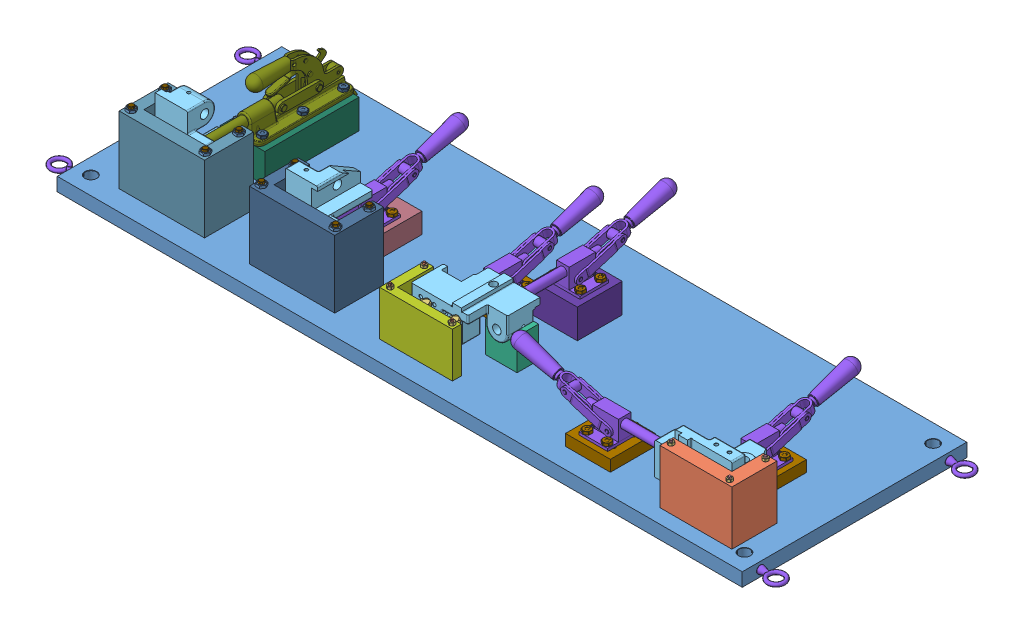
SolidWorks assembly Fixture Assy, configuration Default. Lengths in mm.
Overall size (1638.16 217.94 526.81).
140 component instances, 28 part files, 352 mates.
Components (placement in the parent):
- Base-1: Base [Default] at (275.0152 551.2285 789.288)
- Roller Rest Bracket-1: Roller Rest Bracket [Default] at (1089.0152 646.7285 943.288) x (1 0 0) z (0 -1 0) (hidden)
- U_Block-1: U_Block [Default] at (1090.5152 641.2285 977.288)
- 2336A124_Locating Pin-3: 2336A124_Locating Pin [2336A124] at (1191.5152 644.4833 964.317) x (0 -0.866025 0.5) z (-1 0 0)
- 2336A124_Locating Pin-5: 2336A124_Locating Pin [2336A124] at (1146.7605 666.1995 978.788) x (-0.866025 -0.5 0) z (0 0 -1)
- 2336A124_Locating Pin-6: 2336A124_Locating Pin [2336A124] at (1078.251 666.1995 978.788) x (-0.866025 -0.5 0) z (0 0 -1)
- 3097N13_Press-Fit Locating and Support Button-1: 3097N13_Press-Fit Locating and Support Button [3097N13] at (1105.0152 581.2285 957.288) x (1 0 0) z (0 1 0)
- 3097N13_Press-Fit Locating and Support Button-2: 3097N13_Press-Fit Locating and Support Button [3097N13] at (1025.0152 581.2285 949.288) x (1 0 0) z (0 1 0)
- 3097N13_Press-Fit Locating and Support Button-3: 3097N13_Press-Fit Locating and Support Button [3097N13] at (1060.0152 581.2285 949.288) x (1 0 0) z (0 1 0)
- 2336A124_Locating Pin-8: 2336A124_Locating Pin [2336A124] at (1078.251 621.3039 978.788) x (-0.866025 -0.5 0) z (0 0 -1)
- Roller Rest Bracket-2: Roller Rest Bracket [Default] at (543.5123 671.2285 901.788)
- Vee Block-1: Vee Block [Default] at (605.5123 581.2285 882.288) x (1 0 0) z (0 1 0)
- U - BLock-Operation 2-1: U - BLock-Operation 2 [Default] at (543.5123 631.2285 974.288) x (-1 0 0) z (0 0 1)
- 5222N4_Heavy Duty Reverse-Action Push Toggle Clamp-1: 5222N4_Heavy Duty Reverse-Action Push Toggle Clamp [5222N4] at (1105.0152 641.2285 858.5673)
- Operation 1 Clamp Base-1: Operation 1 Clamp Base [Default] at (1105.0152 581.2285 826.5673)
- 2336A124_Locating Pin-16: 2336A124_Locating Pin [2336A124] at (495.767 671.2285 975.788) x (0.866025 0.5 0) z (0 0 -1)
- 2336A124_Locating Pin-17: 2336A124_Locating Pin [2336A124] at (560.767 671.2285 975.788) x (-0.866025 -0.5 0) z (0 0 -1)
- 2336A124_Locating Pin-18: 2336A124_Locating Pin [2336A124] at (441.0123 662.9738 902.288) x (0 0.866025 -0.5) z (1 0 0)
- 2336A124_Locating Pin-19: 2336A124_Locating Pin [2336A124] at (507.4833 579.7285 924.5428) x (-0.5 0 0.866025) z (0 1 0)
- 5222N4_Heavy Duty Reverse-Action Push Toggle Clamp-4: 5222N4_Heavy Duty Reverse-Action Push Toggle Clamp [5222N4] at (490.0152 641.2285 816.5673)
- Operation 1 Clamp Base-4: Operation 1 Clamp Base [Default] at (490.0152 581.2285 784.5673)
- Roller Rest Bracket-5: Roller Rest Bracket [Default] at (225.0123 675.2285 930.288) x (0 -1 0) z (-1 0 0)
- 3097N13_Press-Fit Locating and Support Button-6: 3097N13_Press-Fit Locating and Support Button [3097N13] at (257.5123 581.2285 969.288) x (0.961852 0 0.273569) z (0 1 0)
- 3097N13_Press-Fit Locating and Support Button-7: 3097N13_Press-Fit Locating and Support Button [3097N13] at (222.5123 581.2285 969.288) x (-0.056694 0 0.998392) z (0 1 0)
- Opeartion 3 BLock-1: Opeartion 3 BLock [Default] at (227.5123 581.2285 994.288) x (-1 0 0) z (0 0 -1)
- 2336A124_Locating Pin-20: 2336A124_Locating Pin [2336A124] at (264.2575 622.2285 965.788) x (-0.866025 0.5 0) z (0 0 -1)
- 2336A124_Locating Pin-22: 2336A124_Locating Pin [2336A124] at (232.748 622.2285 965.788) x (-0.866025 0.5 0) z (0 0 -1)
- 2336A124_Locating Pin-23: 2336A124_Locating Pin [2336A124] at (299.0123 687.2285 941.0333) x (0 -0.5 0.866025) z (-1 0 0)
- 2336A124_Locating Pin-24: 2336A124_Locating Pin [2336A124] at (299.0123 641.2285 941.0333) x (0 -0.5 0.866025) z (-1 0 0)
- Screw Clamp Assy-3: Screw Clamp Assy [Default] at (166.9641 634.1162 934.4665) x (0 0 1) z (-1 0 0) size (29.27 29.27 49.45)
  - 6214K44_Comfort-Grip Plastic Ribbed Knob-1: 6214K44_Comfort-Grip Plastic Ribbed Knob [6214K44] at (9.8216 24.1124 25.0925)
  - 9540K709_Unthreaded Bumper-1: 9540K709_Unthreaded Bumper [9540K709] at (9.5892 24.1617 4.3416) x (0.978178 -0.207769 0) z (-0.207769 -0.978178 0)
- 5222N4_Heavy Duty Reverse-Action Push Toggle Clamp-5: 5222N4_Heavy Duty Reverse-Action Push Toggle Clamp [5222N4] at (218.0152 661.2285 845.5673)
- Operation 3 Clamp Base-5: Operation 3 Clamp Base [Default] at (218.0152 581.2285 795.5673)
- Opeartion 4 BLock-2: Opeartion 4 BLock [Default] at (-62.4877 581.2285 994.288) x (-1 0 0) z (0 0 -1)
- Roller Rest Bracket-6: Roller Rest Bracket [Default] at (-64.9877 675.2285 930.288) x (0 1 0) z (1 0 0)
- 2336A124_Locating Pin-25: 2336A124_Locating Pin [2336A124] at (-96.4877 667.9738 965.788) x (-0.5 -0.866025 0) z (0 0 -1)
- 2336A124_Locating Pin-26: 2336A124_Locating Pin [2336A124] at (-28.4877 667.9738 965.788) x (-0.5 -0.866025 0) z (0 0 -1)
- 2336A124_Locating Pin-27: 2336A124_Locating Pin [2336A124] at (-33.4877 622.9738 965.788) x (-0.5 -0.866025 0) z (0 0 -1)
- 2336A124_Locating Pin-28: 2336A124_Locating Pin [2336A124] at (196.9038 690.4475 965.788) x (-0.923728 -0.383049 0) z (0 0 -1)
- 2336A124_Locating Pin-29: 2336A124_Locating Pin [2336A124] at (9.0123 701.2285 940.288) x (0 -0.998687 -0.051226) z (-1 0 0)
- 2336A124_Locating Pin-30: 2336A124_Locating Pin [2336A124] at (9.0123 631.2285 934.288) x (0 0 1) z (-1 0 0)
- 3097N13_Press-Fit Locating and Support Button-8: 3097N13_Press-Fit Locating and Support Button [3097N13] at (-62.4877 581.2285 934.288) x (1 0 0) z (0 1 0)
- 3097N13_Press-Fit Locating and Support Button-9: 3097N13_Press-Fit Locating and Support Button [3097N13] at (-65.4877 581.2285 909.288) x (1 0 0) z (0 1 0)
- 3097N13_Press-Fit Locating and Support Button-10: 3097N13_Press-Fit Locating and Support Button [3097N13] at (-22.4877 581.2285 934.288) x (1 0 0) z (0 1 0)
- Op 4 Clamp base-6: Op 4 Clamp base [Default] at (-51.9848 581.2285 720.5206)
- 6124A13_Toggle Clamp with Locking Handle-6: 6124A13_Toggle Clamp with Locking Handle [6124A13] at (-51.9848 646.2285 930.288)
- Screw Clamp Assy-4: Screw Clamp Assy [Default] at (-123.0359 669.0512 925.8337) x (0 -0.292948 0.956128) z (-1 0 0) size (29.27 29.27 49.45)
  - 6214K44_Comfort-Grip Plastic Ribbed Knob-1: 6214K44_Comfort-Grip Plastic Ribbed Knob [6214K44] at (9.8216 24.1124 25.0925)
  - 9540K709_Unthreaded Bumper-1: 9540K709_Unthreaded Bumper [9540K709] at (9.5892 24.1617 4.3416) x (0.978178 -0.207769 0) z (-0.207769 -0.978178 0)
- Operation 1 Clamp Base-7: Operation 1 Clamp Base [Default] at (886.2945 581.2285 944.288)
- 5222N4_Heavy Duty Reverse-Action Push Toggle Clamp-7: 5222N4_Heavy Duty Reverse-Action Push Toggle Clamp [5222N4] at (918.2945 641.2285 944.288) x (0 0 -1) z (1 0 0)
- 5222N4_Heavy Duty Reverse-Action Push Toggle Clamp-8: 5222N4_Heavy Duty Reverse-Action Push Toggle Clamp [5222N4] at (596.0152 681.2285 759.5673)
- Operation 2 Clamp Base-8: Operation 2 Clamp Base [Default] at (596.0152 581.2285 727.5673)
- 93516A178_Bronze Hex Head Screw-2: 93516A178_Bronze Hex Head Screw [93516A178] at (310.0123 551.2285 904.813) x (0.866025 0 -0.5) z (0 -1 0)
- 93516A178_Bronze Hex Head Screw-3: 93516A178_Bronze Hex Head Screw [93516A178] at (-144.9877 551.2285 979.763) x (0.866025 0 0.5) z (0 -1 0)
- 93516A178_Bronze Hex Head Screw-4: 93516A178_Bronze Hex Head Screw [93516A178] at (145.0123 551.2285 904.813) x (0.866025 0 0.5) z (0 -1 0)
- 93516A178_Bronze Hex Head Screw-5: 93516A178_Bronze Hex Head Screw [93516A178] at (310.0123 551.2285 979.763) x (0.866025 0 0.5) z (0 -1 0)
- 93516A178_Bronze Hex Head Screw-6: 93516A178_Bronze Hex Head Screw [93516A178] at (20.0123 551.2285 979.763) x (0.866025 0 -0.5) z (0 -1 0)
- 93516A178_Bronze Hex Head Screw-7: 93516A178_Bronze Hex Head Screw [93516A178] at (145.0123 551.2285 979.763) x (0.866025 0 0.5) z (0 -1 0)
- 93516A178_Bronze Hex Head Screw-8: 93516A178_Bronze Hex Head Screw [93516A178] at (20.0123 551.2285 904.813) x (0.866025 0 -0.5) z (0 -1 0)
- 93516A178_Bronze Hex Head Screw-9: 93516A178_Bronze Hex Head Screw [93516A178] at (-144.9877 551.2285 904.813) x (0.866025 0 -0.5) z (0 -1 0)
- 98886A736_High-Strength High-Temperature PEEK Hex Nut-2: 98886A736_High-Strength High-Temperature PEEK Hex Nut [98886A736] at (310.0123 734.4035 904.813)
- 98886A736_High-Strength High-Temperature PEEK Hex Nut-3: 98886A736_High-Strength High-Temperature PEEK Hex Nut [98886A736] at (310.0123 734.4035 979.763) x (-0.837169 0 -0.546944) z (-0.546944 0 0.837169)
- 98886A736_High-Strength High-Temperature PEEK Hex Nut-4: 98886A736_High-Strength High-Temperature PEEK Hex Nut [98886A736] at (145.0123 734.4035 979.763) x (0.837169 0 0.546944) z (0.546944 0 -0.837169)
- 98886A736_High-Strength High-Temperature PEEK Hex Nut-5: 98886A736_High-Strength High-Temperature PEEK Hex Nut [98886A736] at (145.0123 734.4035 904.813) x (-0.837169 0 -0.546944) z (-0.546944 0 0.837169)
- 98886A736_High-Strength High-Temperature PEEK Hex Nut-6: 98886A736_High-Strength High-Temperature PEEK Hex Nut [98886A736] at (-144.9877 734.4035 979.763) x (-0.837169 0 -0.546944) z (-0.546944 0 0.837169)
- 98886A736_High-Strength High-Temperature PEEK Hex Nut-7: 98886A736_High-Strength High-Temperature PEEK Hex Nut [98886A736] at (-144.9877 734.4035 904.813) x (-0.837169 0 -0.546944) z (-0.546944 0 0.837169)
- 98886A736_High-Strength High-Temperature PEEK Hex Nut-8: 98886A736_High-Strength High-Temperature PEEK Hex Nut [98886A736] at (20.0123 734.4035 979.763) x (-0.837169 0 -0.546944) z (-0.546944 0 0.837169)
- 98886A736_High-Strength High-Temperature PEEK Hex Nut-9: 98886A736_High-Strength High-Temperature PEEK Hex Nut [98886A736] at (20.0123 734.4035 904.813) x (-0.837169 0 -0.546944) z (-0.546944 0 0.837169)
- 91268A514_High-Strength Grade 8 Steel Hex Head Screw-1: 91268A514_High-Strength Grade 8 Steel Hex Head Screw [91268A514] at (432.5123 619.0942 904.8443) x (0 1 0) z (0.866025 0 -0.5)
- 91268A514_High-Strength Grade 8 Steel Hex Head Screw-2: 91268A514_High-Strength Grade 8 Steel Hex Head Screw [91268A514] at (435.5615 619.0942 983.7318) x (0 1 0) z (0 0 1)
- 91268A514_High-Strength Grade 8 Steel Hex Head Screw-3: 91268A514_High-Strength Grade 8 Steel Hex Head Screw [91268A514] at (573.956 619.0942 984.288) x (0 1 0) z (-0.5 0 0.866025)
- 95462A029_Medium-Strength Steel Hex Nut-1: 95462A029_Medium-Strength Steel Hex Nut [95462A029] at (435.5615 684.0067 983.7318) x (1 0 0) z (0 -1 0)
- 95462A029_Medium-Strength Steel Hex Nut-2: 95462A029_Medium-Strength Steel Hex Nut [95462A029] at (432.5123 684.0067 904.8443) x (0.837169 0 0.546944) z (0 -1 0)
- 95462A029_Medium-Strength Steel Hex Nut-4: 95462A029_Medium-Strength Steel Hex Nut [95462A029] at (573.956 684.0067 984.288) x (1 0 0) z (0 -1 0)
- 91251A562_Black-Oxide Alloy Steel Socket Head Screw-1: 91251A562_Black-Oxide Alloy Steel Socket Head Screw [91251A562] at (1205.0152 627.4285 997.288) x (0.990541 0 0.13722) z (0 -1 0)
- 91251A562_Black-Oxide Alloy Steel Socket Head Screw-2: 91251A562_Black-Oxide Alloy Steel Socket Head Screw [91251A562] at (1205.0152 627.4285 917.288) x (1 0 0) z (0 -1 0)
- 91251A562_Black-Oxide Alloy Steel Socket Head Screw-3: 91251A562_Black-Oxide Alloy Steel Socket Head Screw [91251A562] at (1069.5123 627.4285 992.288) x (1 0 0) z (0 -1 0)
- 95462A029_Medium-Strength Steel Hex Nut-5: 95462A029_Medium-Strength Steel Hex Nut [95462A029] at (1069.5123 704.0067 992.288) x (1 0 0) z (0 -1 0)
- 95462A029_Medium-Strength Steel Hex Nut-6: 95462A029_Medium-Strength Steel Hex Nut [95462A029] at (1205.0152 704.0067 997.288) x (1 0 0) z (0 -1 0)
- 95462A029_Medium-Strength Steel Hex Nut-7: 95462A029_Medium-Strength Steel Hex Nut [95462A029] at (1205.0152 704.0067 917.288) x (0.779206 0 -0.626768) z (0 -1 0)
- 91257A550_Zinc Yellow-Chromate Plated Hex Head Screw (1)-1: 91257A550_Zinc Yellow-Chromate Plated Hex Head Screw (1) [91257A550] at (634.5994 574.4457 688.1236) x (0 1 0) z (0 0 1)
- 91257A550_Zinc Yellow-Chromate Plated Hex Head Screw (1)-2: 91257A550_Zinc Yellow-Chromate Plated Hex Head Screw (1) [91257A550] at (557.431 574.4457 688.1236) x (0 1 0) z (0 0 1)
- 91257A550_Zinc Yellow-Chromate Plated Hex Head Screw (1)-3: 91257A550_Zinc Yellow-Chromate Plated Hex Head Screw (1) [91257A550] at (557.431 574.4457 767.0111) x (0 1 0) z (0 0 1)
- 91257A550_Zinc Yellow-Chromate Plated Hex Head Screw (1)-4: 91257A550_Zinc Yellow-Chromate Plated Hex Head Screw (1) [91257A550] at (634.5994 574.4457 767.0111) x (0 1 0) z (0 0 1)
- 91257A550_Zinc Yellow-Chromate Plated Hex Head Screw (1)-5: 91257A550_Zinc Yellow-Chromate Plated Hex Head Screw (1) [91257A550] at (-90.569 574.4457 814.9644) x (0 1 0) z (0.866025 0 0.5)
- 91257A550_Zinc Yellow-Chromate Plated Hex Head Screw (1)-6: 91257A550_Zinc Yellow-Chromate Plated Hex Head Screw (1) [91257A550] at (-13.4006 574.4457 814.9644) x (0 1 0) z (0 0 1)
- 91257A550_Zinc Yellow-Chromate Plated Hex Head Screw (1)-7: 91257A550_Zinc Yellow-Chromate Plated Hex Head Screw (1) [91257A550] at (-90.569 574.4457 626.0769) x (0 1 0) z (0 0 1)
- 91257A550_Zinc Yellow-Chromate Plated Hex Head Screw (1)-8: 91257A550_Zinc Yellow-Chromate Plated Hex Head Screw (1) [91257A550] at (-13.4006 574.4457 626.0769) x (0 1 0) z (0.866025 0 0.5)
- 91257A552_Zinc Yellow-Chromate Plated Hex Head Screw-1: 91257A552_Zinc Yellow-Chromate Plated Hex Head Screw [91257A552] at (179.431 580.7957 835.0111) x (0 1 0) z (0 0 1)
- 91257A552_Zinc Yellow-Chromate Plated Hex Head Screw-2: 91257A552_Zinc Yellow-Chromate Plated Hex Head Screw [91257A552] at (256.5994 580.7957 756.1236) x (0 1 0) z (0 0 1)
- 91257A552_Zinc Yellow-Chromate Plated Hex Head Screw-3: 91257A552_Zinc Yellow-Chromate Plated Hex Head Screw [91257A552] at (256.5994 580.7957 835.0111) x (0 1 0) z (0 0 1)
- 91257A552_Zinc Yellow-Chromate Plated Hex Head Screw-4: 91257A552_Zinc Yellow-Chromate Plated Hex Head Screw [91257A552] at (179.431 580.7957 756.1236) x (0 1 0) z (0 0 1)
- 91257A546_Zinc Yellow-Chromate Plated Hex Head Screw-1: 91257A546_Zinc Yellow-Chromate Plated Hex Head Screw [91257A546] at (528.5994 568.0957 745.1236) x (0 1 0) z (0 0 1)
- 91257A546_Zinc Yellow-Chromate Plated Hex Head Screw-2: 91257A546_Zinc Yellow-Chromate Plated Hex Head Screw [91257A546] at (451.431 568.0957 824.0111) x (0 1 0) z (0 0 1)
- 91257A546_Zinc Yellow-Chromate Plated Hex Head Screw-3: 91257A546_Zinc Yellow-Chromate Plated Hex Head Screw [91257A546] at (528.5994 568.0957 824.0111) x (0 1 0) z (0 0 1)
- 91257A546_Zinc Yellow-Chromate Plated Hex Head Screw-4: 91257A546_Zinc Yellow-Chromate Plated Hex Head Screw [91257A546] at (451.431 568.0957 745.1236) x (0 1 0) z (0 0 1)
- 91257A546_Zinc Yellow-Chromate Plated Hex Head Screw-5: 91257A546_Zinc Yellow-Chromate Plated Hex Head Screw [91257A546] at (847.7103 568.0957 983.7318) x (0 1 0) z (0 0 1)
- 91257A546_Zinc Yellow-Chromate Plated Hex Head Screw-6: 91257A546_Zinc Yellow-Chromate Plated Hex Head Screw [91257A546] at (847.7103 568.0957 904.8443) x (0 1 0) z (0 0 1)
- 91257A546_Zinc Yellow-Chromate Plated Hex Head Screw-7: 91257A546_Zinc Yellow-Chromate Plated Hex Head Screw [91257A546] at (924.8787 568.0957 904.8443) x (0 1 0) z (0 0 1)
- 91257A546_Zinc Yellow-Chromate Plated Hex Head Screw-8: 91257A546_Zinc Yellow-Chromate Plated Hex Head Screw [91257A546] at (924.8787 568.0957 983.7318) x (0 1 0) z (0 0 1)
- 91257A546_Zinc Yellow-Chromate Plated Hex Head Screw-9: 91257A546_Zinc Yellow-Chromate Plated Hex Head Screw [91257A546] at (1143.5994 568.0957 787.1236) x (0 1 0) z (0 0 1)
- 91257A546_Zinc Yellow-Chromate Plated Hex Head Screw-10: 91257A546_Zinc Yellow-Chromate Plated Hex Head Screw [91257A546] at (1143.5994 568.0957 866.0111) x (0 1 0) z (0 0 1)
- 91257A546_Zinc Yellow-Chromate Plated Hex Head Screw-11: 91257A546_Zinc Yellow-Chromate Plated Hex Head Screw [91257A546] at (1066.431 568.0957 866.0111) x (0 1 0) z (0 0 1)
- 91257A546_Zinc Yellow-Chromate Plated Hex Head Screw-12: 91257A546_Zinc Yellow-Chromate Plated Hex Head Screw [91257A546] at (1066.431 568.0957 787.1236) x (0 1 0) z (0 0 1)
- 3014T954_Steel Eyebolt with Shoulder - for Lifting-1: 3014T954_Steel Eyebolt with Shoulder - for Lifting [3014T954] at (1310.3371 566.2285 579.288) x (0 0 -1) z (0 -1 0)
- 91257A550_Zinc Yellow-Chromate Plated Hex Head Screw (1)-9: 91257A550_Zinc Yellow-Chromate Plated Hex Head Screw (1) [91257A550] at (630.5123 574.4457 882.288) x (0 1 0) z (0 0 1)
- 91257A550_Zinc Yellow-Chromate Plated Hex Head Screw (1)-10: 91257A550_Zinc Yellow-Chromate Plated Hex Head Screw (1) [91257A550] at (580.5123 574.4457 882.288) x (0 1 0) z (0 0 1)
- 91310A136_High-Strength Class 10.9 Steel Hex Head Screw-1: 91310A136_High-Strength Class 10.9 Steel Hex Head Screw [91310A136] at (1075.6465 610.0685 804.3423) x (1 0 0) z (0 1 0)
- 91310A136_High-Strength Class 10.9 Steel Hex Head Screw-2: 91310A136_High-Strength Class 10.9 Steel Hex Head Screw [91310A136] at (1075.6465 610.0685 848.7923) x (1 0 0) z (0 1 0)
- 91310A136_High-Strength Class 10.9 Steel Hex Head Screw-3: 91310A136_High-Strength Class 10.9 Steel Hex Head Screw [91310A136] at (1134.384 610.0685 804.3423) x (1 0 0) z (0 1 0)
- 91310A136_High-Strength Class 10.9 Steel Hex Head Screw-4: 91310A136_High-Strength Class 10.9 Steel Hex Head Screw [91310A136] at (1134.384 610.0685 848.7923) x (1 0 0) z (0 1 0)
- 91310A136_High-Strength Class 10.9 Steel Hex Head Screw-5: 91310A136_High-Strength Class 10.9 Steel Hex Head Screw [91310A136] at (566.6465 650.0685 749.7923) x (1 0 0) z (0 1 0)
- 91310A136_High-Strength Class 10.9 Steel Hex Head Screw-6: 91310A136_High-Strength Class 10.9 Steel Hex Head Screw [91310A136] at (566.6465 650.0685 705.3423) x (1 0 0) z (0 1 0)
- 91310A136_High-Strength Class 10.9 Steel Hex Head Screw-7: 91310A136_High-Strength Class 10.9 Steel Hex Head Screw [91310A136] at (625.384 650.0685 749.7923) x (1 0 0) z (0 1 0)
- 91310A136_High-Strength Class 10.9 Steel Hex Head Screw-8: 91310A136_High-Strength Class 10.9 Steel Hex Head Screw [91310A136] at (625.384 650.0685 705.3423) x (1 0 0) z (0 1 0)
- 91310A136_High-Strength Class 10.9 Steel Hex Head Screw-9: 91310A136_High-Strength Class 10.9 Steel Hex Head Screw [91310A136] at (908.5195 610.0685 914.9193) x (1 0 0) z (0 1 0)
- 91310A136_High-Strength Class 10.9 Steel Hex Head Screw-10: 91310A136_High-Strength Class 10.9 Steel Hex Head Screw [91310A136] at (908.5195 610.0685 973.6568) x (1 0 0) z (0 1 0)
- 91310A136_High-Strength Class 10.9 Steel Hex Head Screw-11: 91310A136_High-Strength Class 10.9 Steel Hex Head Screw [91310A136] at (864.0695 610.0685 973.6568) x (1 0 0) z (0 1 0)
- 91310A136_High-Strength Class 10.9 Steel Hex Head Screw-12: 91310A136_High-Strength Class 10.9 Steel Hex Head Screw [91310A136] at (864.0695 610.0685 914.9193) x (1 0 0) z (0 1 0)
- 91310A136_High-Strength Class 10.9 Steel Hex Head Screw-13: 91310A136_High-Strength Class 10.9 Steel Hex Head Screw [91310A136] at (519.384 610.0685 806.7923) x (1 0 0) z (0 1 0)
- 91310A136_High-Strength Class 10.9 Steel Hex Head Screw-14: 91310A136_High-Strength Class 10.9 Steel Hex Head Screw [91310A136] at (519.384 610.0685 762.3423) x (1 0 0) z (0 1 0)
- 91310A136_High-Strength Class 10.9 Steel Hex Head Screw-15: 91310A136_High-Strength Class 10.9 Steel Hex Head Screw [91310A136] at (460.6465 610.0685 762.3423) x (1 0 0) z (0 1 0)
- 91310A136_High-Strength Class 10.9 Steel Hex Head Screw-16: 91310A136_High-Strength Class 10.9 Steel Hex Head Screw [91310A136] at (247.384 630.0685 835.7923) x (1 0 0) z (0 1 0)
- 91310A136_High-Strength Class 10.9 Steel Hex Head Screw-17: 91310A136_High-Strength Class 10.9 Steel Hex Head Screw [91310A136] at (247.384 630.0685 791.3423) x (1 0 0) z (0 1 0)
- 91310A136_High-Strength Class 10.9 Steel Hex Head Screw-18: 91310A136_High-Strength Class 10.9 Steel Hex Head Screw [91310A136] at (460.6465 610.0685 806.7923) x (1 0 0) z (0 1 0)
- 91310A136_High-Strength Class 10.9 Steel Hex Head Screw-19: 91310A136_High-Strength Class 10.9 Steel Hex Head Screw [91310A136] at (188.6465 630.0685 791.3423) x (1 0 0) z (0 1 0)
- 91310A136_High-Strength Class 10.9 Steel Hex Head Screw-20: 91310A136_High-Strength Class 10.9 Steel Hex Head Screw [91310A136] at (188.6465 630.0685 835.7923) x (1 0 0) z (0 1 0)
- 90447A250_High-Strength Class 10.9 Steel Hex Head Screw-1: 90447A250_High-Strength Class 10.9 Steel Hex Head Screw [90447A250] at (-79.0358 655.8805 627.1466) x (0 -1 0) z (0 0 1)
- 90447A250_High-Strength Class 10.9 Steel Hex Head Screw-2: 90447A250_High-Strength Class 10.9 Steel Hex Head Screw [90447A250] at (-79.0358 655.8805 717.5706) x (0 -1 0) z (0 0 1)
- 90447A250_High-Strength Class 10.9 Steel Hex Head Screw-3: 90447A250_High-Strength Class 10.9 Steel Hex Head Screw [90447A250] at (-79.0358 655.8805 807.9946) x (0 -1 0) z (0 0 1)
- 90447A250_High-Strength Class 10.9 Steel Hex Head Screw-4: 90447A250_High-Strength Class 10.9 Steel Hex Head Screw [90447A250] at (-24.9338 655.8805 627.1466) x (0 -1 0) z (0 0 1)
- 90447A250_High-Strength Class 10.9 Steel Hex Head Screw-5: 90447A250_High-Strength Class 10.9 Steel Hex Head Screw [90447A250] at (-24.9338 655.8805 717.5706) x (0 -1 0) z (0 0 1)
- 90447A250_High-Strength Class 10.9 Steel Hex Head Screw-6: 90447A250_High-Strength Class 10.9 Steel Hex Head Screw [90447A250] at (-24.9338 655.8805 807.9946) x (0 -1 0) z (0 0 1)
- Roller Rest Bracket-7: Roller Rest Bracket [Default] at (1089.0152 646.7285 943.288) x (-1 0 0) z (0 1 0)
- 2336A124_Locating Pin-9: 2336A124_Locating Pin [2336A124] at (1191.5152 674.4833 964.317) x (0 -0.866025 0.5) z (-1 0 0)
- 3014T954_Steel Eyebolt with Shoulder - for Lifting-5: 3014T954_Steel Eyebolt with Shoulder - for Lifting [3014T954] at (1310.3371 566.2285 999.288) x (0 0 -1) z (0 -1 0)
- 3014T954_Steel Eyebolt with Shoulder - for Lifting-6: 3014T954_Steel Eyebolt with Shoulder - for Lifting [3014T954] at (-285.7588 566.2285 579.288) x (0 0 1) z (0 -1 0)
- 3014T954_Steel Eyebolt with Shoulder - for Lifting-7: 3014T954_Steel Eyebolt with Shoulder - for Lifting [3014T954] at (-285.7588 566.2285 999.288) x (0 0 1) z (0 -1 0)
Mates (geometry in assembly coordinates):
- Coincident20: coincident anti-aligned: plane of Base-1 through (275.0152 581.2285 789.288) normal (0 1 0); plane of Roller Rest Bracket-2 through (543.5123 581.2285 901.788) normal (0 -1 0)
- Coincident21: coincident anti-aligned: plane of Base-1 through (275.0152 581.2285 789.288) normal (0 1 0); plane of Vee Block-1 through (605.5123 581.2285 882.288) normal (0 -1 0)
- Coincident23: coincident anti-aligned: plane of Base-1 through (275.0152 581.2285 789.288) normal (0 1 0); plane of U - BLock-Operation 2-1 through (543.5123 581.2285 974.288) normal (0 -1 0)
- Coincident24: coincident anti-aligned: plane of Base-1 through (275.0152 581.2285 789.288) normal (0 1 0); plane of 3097N13_Press-Fit Locating and Support Button-1 through (1105.0152 581.2285 949.338) normal (0 -1 0)
- Coincident25: coincident anti-aligned: plane of Base-1 through (275.0152 581.2285 789.288) normal (0 1 0); plane of 3097N13_Press-Fit Locating and Support Button-2 through (1025.0152 581.2285 941.338) normal (0 -1 0)
- Coincident26: coincident anti-aligned: plane of Base-1 through (275.0152 581.2285 789.288) normal (0 1 0); plane of 3097N13_Press-Fit Locating and Support Button-3 through (1060.0152 581.2285 941.338) normal (0 -1 0)
- Coincident27: coincident anti-aligned: plane of Roller Rest Bracket-1 through (1003.0152 589.2285 962.288) normal (0 -1 0); plane of 3097N13_Press-Fit Locating and Support Button-1 through (1105.0152 589.2285 957.288) normal (0 1 0)
- Distance6: distance = 70 mm aligned: plane of Base-1 through (-724.9848 581.2285 1039.288) normal (0 0 1); plane of Roller Rest Bracket-1 through (1115.0077 589.2285 969.288) normal (0 0 1)
- Distance7: distance = 100 mm aligned: plane of Roller Rest Bracket-1 through (1175.0152 704.2285 962.288) normal (1 0 0); plane of Base-1 through (1275.0152 581.2285 539.288) normal (1 0 0)
- Distance9: distance = 82 mm: cylinder of 3097N13_Press-Fit Locating and Support Button-1 through (1105.0152 593.9285 957.288) axis (0 1 0) radius 4; plane of Base-1 through (-724.9848 581.2285 1039.288) normal (0 0 1)
- Distance10: distance = 170 mm: cylinder of 3097N13_Press-Fit Locating and Support Button-1 through (1105.0152 593.9285 957.288) axis (0 1 0) radius 4; plane of Base-1 through (1275.0152 581.2285 539.288) normal (1 0 0)
- Distance11: distance = 90 mm: cylinder of 3097N13_Press-Fit Locating and Support Button-3 through (1060.0152 593.9285 949.288) axis (0 1 0) radius 4; plane of Base-1 through (-724.9848 581.2285 1039.288) normal (0 0 1)
- Distance13: distance = 90 mm: cylinder of 3097N13_Press-Fit Locating and Support Button-2 through (1025.0152 593.9285 949.288) axis (0 1 0) radius 4; plane of Base-1 through (-724.9848 581.2285 1039.288) normal (0 0 1)
- Distance14: distance = 215 mm: cylinder of 3097N13_Press-Fit Locating and Support Button-3 through (1060.0152 593.9285 949.288) axis (0 1 0) radius 4; plane of Base-1 through (1275.0152 581.2285 539.288) normal (1 0 0)
- Distance15: distance = 250 mm: cylinder of 3097N13_Press-Fit Locating and Support Button-2 through (1025.0152 593.9285 949.288) axis (0 1 0) radius 4; plane of Base-1 through (1275.0152 581.2285 539.288) normal (1 0 0)
- Coincident30: coincident anti-aligned: plane of Roller Rest Bracket-1 through (1175.0152 704.2285 962.288) normal (1 0 0); plane of 2336A124_Locating Pin-3 through (1175.0152 644.4833 964.317) normal (-1 0 0)
- Coincident33: coincident anti-aligned: plane of Roller Rest Bracket-1 through (1089.0152 646.7285 962.288) normal (0 0 1); plane of 2336A124_Locating Pin-6 through (1078.251 666.1995 962.288) normal (0 0 -1)
- Coincident34: coincident anti-aligned: plane of Roller Rest Bracket-1 through (1089.0152 646.7285 962.288) normal (0 0 1); plane of 2336A124_Locating Pin-5 through (1146.7605 666.1995 962.288) normal (0 0 -1)
- Coincident35: coincident anti-aligned: plane of Roller Rest Bracket-1 through (1089.0152 646.7285 962.288) normal (0 0 1); plane of 2336A124_Locating Pin-8 through (1078.251 621.3039 962.288) normal (0 0 -1)
- Distance16: distance = 120 mm aligned: plane of 2336A124_Locating Pin-5 through (1155.0152 650.1449 962.288) normal (1 0 0); plane of Base-1 through (1275.0152 581.2285 539.288) normal (1 0 0)
- Distance17: distance = 75 mm: line of 2336A124_Locating Pin-5 through (1147.5213 656.2285 971.288) axis (0 0 1); plane of Base-1 through (275.0152 581.2285 789.288) normal (0 1 0)
- Distance18: distance = 52 mm anti-aligned: plane of 2336A124_Locating Pin-6 through (1086.5057 650.1449 962.288) normal (1 0 0); plane of 2336A124_Locating Pin-5 through (1138.5057 671.8439 962.288) normal (-1 0 0)
- Distance19: distance = 75 mm: line of 2336A124_Locating Pin-6 through (1079.0118 656.2285 971.288) axis (0 0 1); plane of Base-1 through (275.0152 581.2285 789.288) normal (0 1 0)
- Coincident41: coincident aligned: plane of 2336A124_Locating Pin-6 through (1086.5057 650.1449 962.288) normal (1 0 0); plane of 2336A124_Locating Pin-8 through (1086.5057 605.2492 962.288) normal (1 0 0)
- Distance20: distance = 25 mm: line of 2336A124_Locating Pin-6 through (1079.0118 656.2285 971.288) axis (0 0 1); line of 2336A124_Locating Pin-8 through (1077.4901 631.2749 976.888) axis (0 0 -1)
- Distance24: distance = 55 mm anti-aligned: plane of Base-1 through (275.0152 581.2285 789.288) normal (0 1 0); plane of 2336A124_Locating Pin-3 through (1175.0152 636.2285 969.0829) normal (0 -1 0)
- Distance25: distance = 65 mm: line of 2336A124_Locating Pin-3 through (1189.6152 645.2441 974.288) axis (-1 0 0); plane of Base-1 through (-724.9848 581.2285 1039.288) normal (0 0 1)
- Coincident48: coincident anti-aligned: plane of U_Block-1 through (991.0152 701.2285 977.288) normal (0 0 -1); plane of 2336A124_Locating Pin-5 through (1141.7605 674.8598 977.288) normal (0 0 1)
- Coincident49: coincident anti-aligned: plane of U_Block-1 through (1190.0152 701.2285 977.288) normal (-1 0 0); plane of 2336A124_Locating Pin-9 through (1190.0152 679.4833 972.9773) normal (1 0 0)
- Coincident50: coincident anti-aligned: plane of Base-1 through (275.0152 581.2285 789.288) normal (0 1 0); plane of U_Block-1 through (1090.5152 581.2285 977.288) normal (0 -1 0)
- Coincident51: coincident anti-aligned: plane of Base-1 through (275.0152 581.2285 789.288) normal (0 1 0); plane of Operation 1 Clamp Base-1 through (1105.0152 581.2285 826.5673) normal (0 -1 0)
- Distance27: distance = 120 mm aligned: plane of Operation 1 Clamp Base-1 through (1155.0152 606.2285 776.5673) normal (1 0 0); plane of Base-1 through (1275.0152 581.2285 539.288) normal (1 0 0)
- Coincident55: coincident anti-aligned: plane of 5222N4_Heavy Duty Reverse-Action Push Toggle Clamp-1 through (1067.0152 606.2285 794.5673) normal (0 -1 0); plane of Operation 1 Clamp Base-1 through (1105.0152 606.2285 826.5673) normal (0 1 0)
- Width3: width anti-aligned: plane of 5222N4_Heavy Duty Reverse-Action Push Toggle Clamp-1 through (1143.0152 612.2285 858.5673) normal (1 0 0); plane of Operation 1 Clamp Base-1 through (1067.0152 612.2285 858.5673) normal (-1 0 0); plane of 5222N4_Heavy Duty Reverse-Action Push Toggle Clamp-1 through (1055.0152 606.2285 776.5673) normal (-1 0 0); plane of Operation 1 Clamp Base-1 through (1155.0152 606.2285 776.5673) normal (1 0 0)
- Width4: width anti-aligned: plane of 5222N4_Heavy Duty Reverse-Action Push Toggle Clamp-1 through (1143.0152 612.2285 794.5673) normal (0 0 -1); plane of Operation 1 Clamp Base-1 through (1143.0152 612.2285 858.5673) normal (0 0 1); plane of 5222N4_Heavy Duty Reverse-Action Push Toggle Clamp-1 through (1055.0152 606.2285 876.5673) normal (0 0 1); plane of Operation 1 Clamp Base-1 through (1055.0152 606.2285 776.5673) normal (0 0 -1)
- Coincident56: coincident anti-aligned: plane of Roller Rest Bracket-1 through (1089.0152 646.7285 943.288) normal (0 0 -1); plane of 5222N4_Heavy Duty Reverse-Action Push Toggle Clamp-1 through (1105.0152 641.2285 943.288) normal (0 0 1)
- Distance44: distance = 475 mm anti-aligned: plane of U_Block-1 through (1059.5123 701.2285 1007.288) normal (-1 0 0); plane of U - BLock-Operation 2-1 through (584.5123 581.2285 894.288) normal (1 0 0)
- Coincident102: coincident anti-aligned: plane of U - BLock-Operation 2-1 through (644.5123 581.2285 974.288) normal (0 0 -1); plane of 2336A124_Locating Pin-17 through (555.767 679.8888 974.288) normal (0 0 1)
- Coincident104: coincident anti-aligned: plane of U - BLock-Operation 2-1 through (644.5123 581.2285 974.288) normal (0 0 -1); plane of 2336A124_Locating Pin-16 through (500.767 662.5683 974.288) normal (0 0 1)
- Coincident106: coincident anti-aligned: plane of Roller Rest Bracket-2 through (457.5123 690.2285 959.288) normal (0 0 1); plane of 2336A124_Locating Pin-17 through (560.767 671.2285 959.288) normal (0 0 -1)
- Distance45: distance = 90 mm: cylinder of 2336A124_Locating Pin-16 through (495.767 671.2285 992.288) axis (0 0 1) radius 6; plane of Base-1 through (275.0152 581.2285 789.288) normal (0 1 0)
- Distance46: distance = 90 mm: cylinder of 2336A124_Locating Pin-17 through (560.767 671.2285 992.288) axis (0 0 1) radius 6; plane of Base-1 through (275.0152 581.2285 789.288) normal (0 1 0)
- Distance47: distance = 110 mm anti-aligned: plane of 2336A124_Locating Pin-17 through (552.5123 676.8729 959.288) normal (-1 0 0); plane of U - BLock-Operation 2-1 through (442.5123 581.2285 974.288) normal (1 0 0)
- Coincident108: coincident anti-aligned: plane of Roller Rest Bracket-2 through (457.5123 690.2285 844.288) normal (-1 0 0); plane of 2336A124_Locating Pin-18 through (457.5123 662.9738 902.288) normal (1 0 0)
- Coincident109: coincident anti-aligned: plane of U - BLock-Operation 2-1 through (442.5123 581.2285 974.288) normal (1 0 0); plane of 2336A124_Locating Pin-18 through (442.5123 667.9738 910.9483) normal (-1 0 0)
- Distance48: distance = 45 mm anti-aligned: plane of 2336A124_Locating Pin-16 through (487.5123 687.2832 959.288) normal (-1 0 0); plane of U - BLock-Operation 2-1 through (442.5123 581.2285 974.288) normal (1 0 0)
- Width7: width anti-aligned: plane of Roller Rest Bracket-2 through (629.5123 690.2285 844.288) normal (1 0 0); plane of Vee Block-1 through (581.5123 671.2285 857.958) normal (-1 0 0); plane of Roller Rest Bracket-2 through (570.5123 651.2285 858.288) normal (-1 0 0); plane of Vee Block-1 through (640.5123 651.2285 858.288) normal (1 0 0)
- Coincident114: coincident anti-aligned: plane of Base-1 through (275.0152 581.2285 789.288) normal (0 1 0); plane of 2336A124_Locating Pin-19 through (516.1435 581.2285 929.5428) normal (0 -1 0)
- Coincident115: coincident anti-aligned: plane of Roller Rest Bracket-2 through (457.5123 581.2285 916.288) normal (0 0 1); plane of 2336A124_Locating Pin-19 through (491.4286 596.2285 916.288) normal (0 0 -1)
- Distance52: distance = 55 mm: line of 2336A124_Locating Pin-19 through (497.5123 587.2285 923.782) axis (0 -1 0); plane of U - BLock-Operation 2-1 through (442.5123 581.2285 974.288) normal (1 0 0)
- Coincident118: coincident anti-aligned: plane of Base-1 through (275.0152 581.2285 789.288) normal (0 1 0); plane of Operation 1 Clamp Base-4 through (490.0152 581.2285 784.5673) normal (0 -1 0)
- Coincident121: coincident anti-aligned: plane of 5222N4_Heavy Duty Reverse-Action Push Toggle Clamp-4 through (452.0152 606.2285 752.5673) normal (0 -1 0); plane of Operation 1 Clamp Base-4 through (490.0152 606.2285 784.5673) normal (0 1 0)
- Width8: width anti-aligned: plane of Operation 1 Clamp Base-4 through (440.0152 606.2285 734.5673) normal (-1 0 0); plane of 5222N4_Heavy Duty Reverse-Action Push Toggle Clamp-4 through (540.0152 606.2285 734.5673) normal (1 0 0); plane of Operation 1 Clamp Base-4 through (528.0152 612.2285 816.5673) normal (1 0 0); plane of 5222N4_Heavy Duty Reverse-Action Push Toggle Clamp-4 through (452.0152 612.2285 816.5673) normal (-1 0 0)
- Width9: width anti-aligned: plane of 5222N4_Heavy Duty Reverse-Action Push Toggle Clamp-4 through (528.0152 612.2285 752.5673) normal (0 0 -1); plane of Operation 1 Clamp Base-4 through (528.0152 612.2285 816.5673) normal (0 0 1); plane of 5222N4_Heavy Duty Reverse-Action Push Toggle Clamp-4 through (440.0152 606.2285 834.5673) normal (0 0 1); plane of Operation 1 Clamp Base-4 through (440.0152 606.2285 734.5673) normal (0 0 -1)
- Coincident122: coincident anti-aligned: plane of Roller Rest Bracket-2 through (511.5123 671.2285 901.288) normal (0 0 -1); plane of 5222N4_Heavy Duty Reverse-Action Push Toggle Clamp-4 through (490.0152 641.2285 901.288) normal (0 0 1)
- Distance55: distance = 515 mm anti-aligned: plane of Operation 1 Clamp Base-4 through (540.0152 606.2285 734.5673) normal (1 0 0); plane of Operation 1 Clamp Base-1 through (1055.0152 606.2285 776.5673) normal (-1 0 0)
- Coincident126: coincident anti-aligned: plane of Base-1 through (275.0152 581.2285 789.288) normal (0 1 0); plane of 3097N13_Press-Fit Locating and Support Button-6 through (259.6871 581.2285 961.6413) normal (0 -1 0)
- Coincident127: coincident anti-aligned: plane of Base-1 through (275.0152 581.2285 789.288) normal (0 1 0); plane of 3097N13_Press-Fit Locating and Support Button-7 through (230.4495 581.2285 969.7388) normal (0 -1 0)
- Distance56: distance = 70 mm: cylinder of 3097N13_Press-Fit Locating and Support Button-6 through (257.5123 593.9285 969.288) axis (0 1 0) radius 4; plane of Base-1 through (-724.9848 581.2285 1039.288) normal (0 0 1)
- Distance57: distance = 70 mm: plane of Base-1 through (-724.9848 581.2285 1039.288) normal (0 0 1); cylinder of 3097N13_Press-Fit Locating and Support Button-7 through (222.5123 593.9285 969.288) axis (0 1 0) radius 4
- Coincident128: coincident anti-aligned: plane of Base-1 through (275.0152 581.2285 789.288) normal (0 1 0); plane of Opeartion 3 BLock-1 through (227.5123 581.2285 994.288) normal (0 -1 0)
- Coincident130: coincident anti-aligned: plane of Roller Rest Bracket-5 through (282.5123 589.2285 949.288) normal (0 -1 0); plane of 3097N13_Press-Fit Locating and Support Button-6 through (257.5123 589.2285 969.288) normal (0 1 0)
- Coincident131: coincident anti-aligned: plane of Opeartion 3 BLock-1 through (157.5123 731.2285 964.288) normal (0 0 -1); plane of 2336A124_Locating Pin-20 through (269.2575 630.8888 964.288) normal (0 0 1)
- Coincident133: coincident anti-aligned: plane of Opeartion 3 BLock-1 through (157.5123 731.2285 964.288) normal (0 0 -1); plane of 2336A124_Locating Pin-22 through (237.748 630.8888 964.288) normal (0 0 1)
- Coincident135: coincident anti-aligned: plane of Roller Rest Bracket-5 through (225.0123 675.2285 949.288) normal (0 0 1); plane of 2336A124_Locating Pin-20 through (264.2575 622.2285 949.288) normal (0 0 -1)
- Coincident137: coincident anti-aligned: plane of Opeartion 3 BLock-1 through (297.5123 731.2285 964.288) normal (-1 0 0); plane of 2336A124_Locating Pin-23 through (297.5123 695.8888 946.0333) normal (1 0 0)
- Coincident138: coincident anti-aligned: plane of Opeartion 3 BLock-1 through (297.5123 731.2285 964.288) normal (-1 0 0); plane of 2336A124_Locating Pin-24 through (297.5123 649.8888 946.0333) normal (1 0 0)
- Coincident139: coincident anti-aligned: plane of Roller Rest Bracket-5 through (282.5123 761.2285 949.288) normal (1 0 0); plane of 2336A124_Locating Pin-24 through (282.5123 641.2285 941.0333) normal (-1 0 0)
- Coincident140: coincident anti-aligned: plane of Roller Rest Bracket-5 through (167.5123 761.2285 949.288) normal (-1 0 0); plane of Screw Clamp Assy-3/9540K709_Unthreaded Bumper-1 through (167.5123 658.2285 944.288) normal (1 0 0)
- Distance58: distance = 100 mm anti-aligned: plane of U - BLock-Operation 2-1 through (422.5123 581.2285 894.288) normal (-1 0 0); plane of Opeartion 3 BLock-1 through (322.5123 731.2285 885.288) normal (1 0 0)
- Distance59: distance = 20 mm: plane of Opeartion 3 BLock-1 through (157.5123 731.2285 964.288) normal (0 0 -1); cylinder of Screw Clamp Assy-3/9540K709_Unthreaded Bumper-1 through (163.4163 658.2285 944.288) axis (-1 0 0) radius 7.5813
- Distance60: distance = 77 mm: plane of Base-1 through (275.0152 581.2285 789.288) normal (0 1 0); cylinder of Screw Clamp Assy-3/9540K709_Unthreaded Bumper-1 through (163.4163 658.2285 944.288) axis (-1 0 0) radius 7.5813
- Distance61: distance = 15 mm anti-aligned: plane of 2336A124_Locating Pin-23 through (282.5123 692.8729 949.288) normal (0 0 1); plane of Opeartion 3 BLock-1 through (157.5123 731.2285 964.288) normal (0 0 -1)
- Distance62: distance = 100 mm: cylinder of 2336A124_Locating Pin-23 through (315.5123 687.2285 941.0333) axis (1 0 0) radius 6; plane of Base-1 through (275.0152 581.2285 789.288) normal (0 1 0)
- Coincident144: coincident aligned: plane of 2336A124_Locating Pin-23 through (282.5123 692.8729 949.288) normal (0 0 1); plane of 2336A124_Locating Pin-24 through (282.5123 646.8729 949.288) normal (0 0 1)
- Distance63: distance = 60 mm: cylinder of 2336A124_Locating Pin-24 through (315.5123 641.2285 941.0333) axis (1 0 0) radius 6; plane of Base-1 through (275.0152 581.2285 789.288) normal (0 1 0)
- Distance64: distance = 25 mm anti-aligned: plane of Opeartion 3 BLock-1 through (297.5123 731.2285 964.288) normal (-1 0 0); plane of 2336A124_Locating Pin-20 through (272.5123 627.8729 949.288) normal (1 0 0)
- Distance65: distance = 35 mm: cylinder of 2336A124_Locating Pin-20 through (264.2575 622.2285 982.288) axis (0 0 1) radius 6; plane of Base-1 through (275.0152 581.2285 789.288) normal (0 1 0)
- Distance66: distance = 15 mm anti-aligned: plane of 2336A124_Locating Pin-20 through (256.0028 626.9944 949.288) normal (-1 0 0); plane of 2336A124_Locating Pin-22 through (241.0028 627.8729 949.288) normal (1 0 0)
- Distance67: distance = 35 mm: cylinder of 2336A124_Locating Pin-22 through (232.748 622.2285 982.288) axis (0 0 1) radius 6; plane of Base-1 through (275.0152 581.2285 789.288) normal (0 1 0)
- Distance68: distance = 40 mm: cylinder of 3097N13_Press-Fit Locating and Support Button-6 through (257.5123 593.9285 969.288) axis (0 1 0) radius 4; plane of Opeartion 3 BLock-1 through (297.5123 731.2285 964.288) normal (-1 0 0)
- Distance69: distance = 65 mm: cylinder of 3097N13_Press-Fit Locating and Support Button-7 through (222.5123 593.9285 969.288) axis (0 1 0) radius 4; plane of Opeartion 3 BLock-1 through (157.5123 731.2285 885.288) normal (1 0 0)
- Coincident145: coincident anti-aligned: plane of Base-1 through (275.0152 581.2285 789.288) normal (0 1 0); plane of Operation 3 Clamp Base-5 through (218.0152 581.2285 795.5673) normal (0 -1 0)
- Coincident146: coincident anti-aligned: plane of 5222N4_Heavy Duty Reverse-Action Push Toggle Clamp-5 through (180.0152 626.2285 781.5673) normal (0 -1 0); plane of Operation 3 Clamp Base-5 through (218.0152 626.2285 795.5673) normal (0 1 0)
- Width10: width anti-aligned: plane of 5222N4_Heavy Duty Reverse-Action Push Toggle Clamp-5 through (180.0152 632.2285 845.5673) normal (-1 0 0); plane of 5222N4_Heavy Duty Reverse-Action Push Toggle Clamp-5 through (256.0152 632.2285 845.5673) normal (1 0 0); plane of Operation 3 Clamp Base-5 through (268.0152 626.2285 745.5673) normal (1 0 0); plane of Operation 3 Clamp Base-5 through (168.0152 626.2285 745.5673) normal (-1 0 0)
- Coincident147: coincident anti-aligned: plane of Roller Rest Bracket-5 through (225.0123 675.2285 930.288) normal (0 0 -1); plane of 5222N4_Heavy Duty Reverse-Action Push Toggle Clamp-5 through (218.0152 661.2285 930.288) normal (0 0 1)
- Coincident148: coincident aligned: plane of 5222N4_Heavy Duty Reverse-Action Push Toggle Clamp-5 through (256.0152 632.2285 845.5673) normal (0 0 1); plane of Operation 3 Clamp Base-5 through (168.0152 626.2285 845.5673) normal (0 0 1)
- Distance70: distance = 172 mm anti-aligned: plane of Operation 3 Clamp Base-5 through (268.0152 626.2285 745.5673) normal (1 0 0); plane of Operation 1 Clamp Base-4 through (440.0152 606.2285 734.5673) normal (-1 0 0)
- Coincident150: coincident anti-aligned: plane of Base-1 through (275.0152 581.2285 789.288) normal (0 1 0); plane of Opeartion 4 BLock-2 through (-62.4877 581.2285 994.288) normal (0 -1 0)
- Coincident151: coincident aligned: plane of Opeartion 3 BLock-1 through (322.5123 731.2285 994.288) normal (0 0 1); plane of Opeartion 4 BLock-2 through (32.5123 731.2285 994.288) normal (0 0 1)
- Distance71: distance = 100 mm anti-aligned: plane of Opeartion 4 BLock-2 through (32.5123 731.2285 885.288) normal (1 0 0); plane of Opeartion 3 BLock-1 through (132.5123 731.2285 994.288) normal (-1 0 0)
- Coincident153: coincident anti-aligned: plane of Opeartion 4 BLock-2 through (-132.4877 731.2285 964.288) normal (0 0 -1); plane of 2336A124_Locating Pin-25 through (-105.148 672.9738 964.288) normal (0 0 1)
- Coincident154: coincident anti-aligned: plane of Opeartion 4 BLock-2 through (-132.4877 731.2285 964.288) normal (0 0 -1); plane of 2336A124_Locating Pin-26 through (-37.148 672.9738 964.288) normal (0 0 1)
- Coincident155: coincident anti-aligned: plane of Opeartion 4 BLock-2 through (-132.4877 731.2285 964.288) normal (0 0 -1); plane of 2336A124_Locating Pin-28 through (193.0733 699.6847 964.288) normal (0 0 1)
- Coincident156: coincident anti-aligned: plane of Opeartion 4 BLock-2 through (-132.4877 731.2285 964.288) normal (0 0 -1); plane of 2336A124_Locating Pin-27 through (-42.148 627.9738 964.288) normal (0 0 1)
- Coincident158: coincident anti-aligned: plane of Opeartion 4 BLock-2 through (7.5123 731.2285 964.288) normal (-1 0 0); plane of 2336A124_Locating Pin-29 through (7.5123 700.7163 950.2749) normal (1 0 0)
- Coincident159: coincident anti-aligned: plane of Opeartion 4 BLock-2 through (7.5123 731.2285 964.288) normal (-1 0 0); plane of 2336A124_Locating Pin-30 through (7.5123 641.2285 934.288) normal (1 0 0)
- Coincident160: coincident anti-aligned: plane of Roller Rest Bracket-6 through (-7.4877 589.2285 949.288) normal (1 0 0); plane of 2336A124_Locating Pin-29 through (-7.4877 701.2285 940.288) normal (-1 0 0)
- Coincident161: coincident anti-aligned: plane of Roller Rest Bracket-6 through (-64.9877 675.2285 949.288) normal (0 0 1); plane of 2336A124_Locating Pin-25 through (-96.4877 667.9738 949.288) normal (0 0 -1)
- Distance73: distance = 55 mm aligned: plane of 2336A124_Locating Pin-25 through (-102.1321 676.2285 949.288) normal (0 1 0); plane of Opeartion 4 BLock-2 through (-62.4877 731.2285 994.288) normal (0 1 0)
- Distance74: distance = 55 mm aligned: plane of 2336A124_Locating Pin-26 through (-34.1321 676.2285 949.288) normal (0 1 0); plane of Opeartion 4 BLock-2 through (-62.4877 731.2285 994.288) normal (0 1 0)
- Distance75: distance = 30 mm anti-aligned: cylinder of 2336A124_Locating Pin-25 through (-96.4877 667.9738 982.288) axis (0 0 1) radius 6; plane of Opeartion 4 BLock-2 through (-132.4877 731.2285 885.288) normal (1 0 0)
- Distance76: distance = 30 mm anti-aligned: cylinder of 2336A124_Locating Pin-26 through (-28.4877 667.9738 982.288) axis (0 0 1) radius 6; plane of Opeartion 4 BLock-2 through (7.5123 731.2285 964.288) normal (-1 0 0)
- Distance77: distance = 100 mm aligned: plane of 2336A124_Locating Pin-27 through (-39.1321 631.2285 949.288) normal (0 1 0); plane of Opeartion 4 BLock-2 through (-62.4877 731.2285 994.288) normal (0 1 0)
- Distance78: distance = 35 mm: cylinder of 2336A124_Locating Pin-27 through (-33.4877 622.9738 982.288) axis (0 0 1) radius 6; plane of Opeartion 4 BLock-2 through (7.5123 731.2285 964.288) normal (-1 0 0)
- Coincident165: coincident anti-aligned: plane of Base-1 through (275.0152 581.2285 789.288) normal (0 1 0); plane of 3097N13_Press-Fit Locating and Support Button-10 through (-22.4877 581.2285 926.338) normal (0 -1 0)
- Coincident166: coincident anti-aligned: plane of Base-1 through (275.0152 581.2285 789.288) normal (0 1 0); plane of 3097N13_Press-Fit Locating and Support Button-9 through (-65.4877 581.2285 901.338) normal (0 -1 0)
- Coincident167: coincident anti-aligned: plane of Base-1 through (275.0152 581.2285 789.288) normal (0 1 0); plane of 3097N13_Press-Fit Locating and Support Button-8 through (-62.4877 581.2285 926.338) normal (0 -1 0)
- Distance79: distance = 30 mm: cylinder of 3097N13_Press-Fit Locating and Support Button-8 through (-62.4877 593.9285 934.288) axis (0 1 0) radius 4; plane of Opeartion 4 BLock-2 through (-132.4877 731.2285 964.288) normal (0 0 -1)
- Distance80: distance = 70 mm: cylinder of 3097N13_Press-Fit Locating and Support Button-8 through (-62.4877 593.9285 934.288) axis (0 1 0) radius 4; plane of Opeartion 4 BLock-2 through (-132.4877 731.2285 885.288) normal (1 0 0)
- Distance81: distance = 30 mm: cylinder of 3097N13_Press-Fit Locating and Support Button-10 through (-22.4877 593.9285 934.288) axis (0 1 0) radius 4; plane of Opeartion 4 BLock-2 through (-132.4877 731.2285 964.288) normal (0 0 -1)
- Distance82: distance = 30 mm: cylinder of 3097N13_Press-Fit Locating and Support Button-10 through (-22.4877 593.9285 934.288) axis (0 1 0) radius 4; plane of Opeartion 4 BLock-2 through (7.5123 731.2285 964.288) normal (-1 0 0)
- Distance83: distance = 55 mm: plane of Opeartion 4 BLock-2 through (-132.4877 731.2285 964.288) normal (0 0 -1); cylinder of 3097N13_Press-Fit Locating and Support Button-9 through (-65.4877 593.9285 909.288) axis (0 1 0) radius 4
- Distance84: distance = 67 mm: cylinder of 3097N13_Press-Fit Locating and Support Button-9 through (-65.4877 593.9285 909.288) axis (0 1 0) radius 4; plane of Opeartion 4 BLock-2 through (-132.4877 731.2285 885.288) normal (1 0 0)
- Distance85: distance = 24 mm: plane of Opeartion 4 BLock-2 through (-132.4877 731.2285 964.288) normal (0 0 -1); cylinder of 2336A124_Locating Pin-29 through (25.5123 701.2285 940.288) axis (1 0 0) radius 6
- Distance87: distance = 120 mm: cylinder of 2336A124_Locating Pin-29 through (25.5123 701.2285 940.288) axis (1 0 0) radius 6; plane of Base-1 through (275.0152 581.2285 789.288) normal (0 1 0)
- Distance88: distance = 50 mm: cylinder of 2336A124_Locating Pin-30 through (25.5123 631.2285 934.288) axis (1 0 0) radius 6; plane of Base-1 through (275.0152 581.2285 789.288) normal (0 1 0)
- Distance89: distance = 30 mm: cylinder of 2336A124_Locating Pin-30 through (25.5123 631.2285 934.288) axis (1 0 0) radius 6; plane of Opeartion 4 BLock-2 through (-132.4877 731.2285 964.288) normal (0 0 -1)
- Coincident168: coincident anti-aligned: plane of Roller Rest Bracket-6 through (-122.4877 589.2285 949.288) normal (0 -1 0); plane of 3097N13_Press-Fit Locating and Support Button-10 through (-22.4877 589.2285 934.288) normal (0 1 0)
- Coincident169: coincident anti-aligned: plane of Base-1 through (275.0152 581.2285 789.288) normal (0 1 0); plane of Op 4 Clamp base-6 through (-51.9848 581.2285 720.5206) normal (0 -1 0)
- Coincident173: coincident anti-aligned: plane of Roller Rest Bracket-6 through (-64.9877 675.2285 930.288) normal (0 0 -1); plane of 6124A13_Toggle Clamp with Locking Handle-6 through (-51.9848 677.9785 930.288) normal (0 0 1)
- Coincident174: coincident anti-aligned: plane of Op 4 Clamp base-6 through (-51.9848 646.2285 720.5206) normal (0 1 0); plane of 6124A13_Toggle Clamp with Locking Handle-6 through (-90.0848 646.2285 600.9182) normal (0 -1 0)
- Coincident177: coincident: plane of Op 4 Clamp base-6 through (-101.9848 646.2285 825.5206) normal (0 0 1); line of 6124A13_Toggle Clamp with Locking Handle-6 through (-26.5848 650.2925 825.5206) axis (-1 0 0)
- Width14: width anti-aligned: plane of Op 4 Clamp base-6 through (-101.9848 646.2285 615.5206) normal (-1 0 0); plane of Op 4 Clamp base-6 through (-1.9848 646.2285 615.5206) normal (1 0 0); plane of 6124A13_Toggle Clamp with Locking Handle-6 through (-34.535 677.292 673.116) normal (1 0 0); plane of 6124A13_Toggle Clamp with Locking Handle-6 through (-69.4346 677.9785 752.488) normal (-1 0 0)
- Coincident178: coincident anti-aligned: plane of Roller Rest Bracket-6 through (-122.4877 589.2285 949.288) normal (-1 0 0); plane of Screw Clamp Assy-4/9540K709_Unthreaded Bumper-1 through (-122.4877 689.2285 942.288) normal (1 0 0)
- Distance90: distance = 22 mm: cylinder of Screw Clamp Assy-4/9540K709_Unthreaded Bumper-1 through (-126.5837 689.2285 942.288) axis (-1 0 0) radius 7.5813; plane of Opeartion 4 BLock-2 through (-132.4877 731.2285 964.288) normal (0 0 -1)
- Distance91: distance = 42 mm: cylinder of Screw Clamp Assy-4/9540K709_Unthreaded Bumper-1 through (-126.5837 689.2285 942.288) axis (-1 0 0) radius 7.5813; plane of Opeartion 4 BLock-2 through (-62.4877 731.2285 994.288) normal (0 1 0)
- Distance92: distance = 170 mm anti-aligned: plane of Op 4 Clamp base-6 through (-1.9848 646.2285 615.5206) normal (1 0 0); plane of Operation 3 Clamp Base-5 through (168.0152 626.2285 745.5673) normal (-1 0 0)
- Coincident181: coincident anti-aligned: plane of Base-1 through (275.0152 581.2285 789.288) normal (0 1 0); plane of Operation 1 Clamp Base-7 through (886.2945 581.2285 944.288) normal (0 -1 0)
- Width15: width anti-aligned: plane of Operation 1 Clamp Base-7 through (836.2945 606.2285 894.288) normal (0 0 -1); plane of Operation 1 Clamp Base-7 through (836.2945 606.2285 994.288) normal (0 0 1); plane of 5222N4_Heavy Duty Reverse-Action Push Toggle Clamp-7 through (918.2945 612.2285 982.288) normal (0 0 1); plane of 5222N4_Heavy Duty Reverse-Action Push Toggle Clamp-7 through (918.2945 612.2285 906.288) normal (0 0 -1)
- Width16: width anti-aligned: plane of 5222N4_Heavy Duty Reverse-Action Push Toggle Clamp-7 through (854.2945 612.2285 906.288) normal (-1 0 0); plane of 5222N4_Heavy Duty Reverse-Action Push Toggle Clamp-7 through (918.2945 612.2285 906.288) normal (1 0 0); plane of Operation 1 Clamp Base-7 through (936.2945 606.2285 894.288) normal (1 0 0); plane of Operation 1 Clamp Base-7 through (836.2945 606.2285 894.288) normal (-1 0 0)
